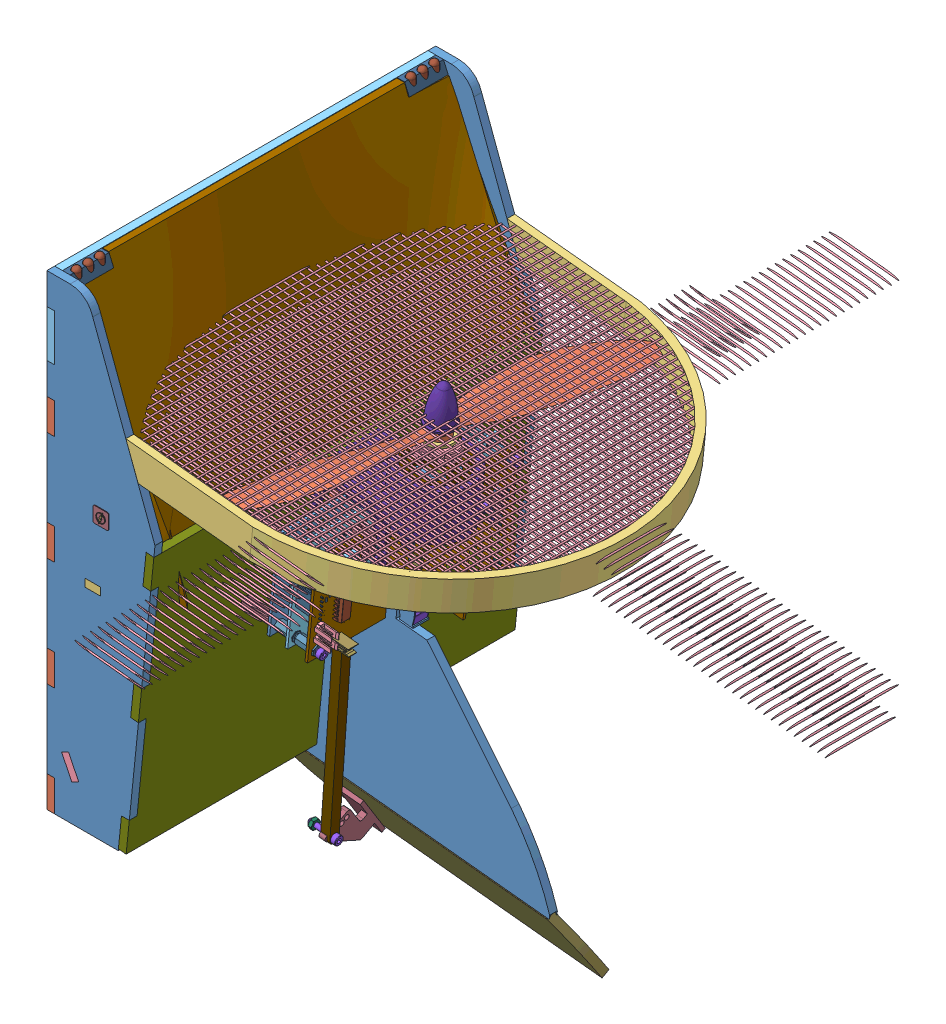
SolidWorks assembly AssTotaleSimu2, configuration Défaut. Lengths in mm. (continued)
Components (placement in the parent): (continued)
- AssStructSimu-1: AssStructSimu [Défaut] at (-125.7658 -1.8483 624.6548) x (1 0 0) z (0 0 -1) size (253.25 324.59 251.6) (continued)
  - AssProtec-1: AssProtec [Défaut] at (86.6746 190.4649 284.6351) x (0 0 -1) z (0.101852 -0.9948 0) size (250 237.46 20) (continued)
    - AssGrillage-2: AssGrillage [Défaut] at (339.6086 -132.5428 241.6839) x (0 0 1) z (-1 0 0) size (2.02 237.05 250) (continued)
      - barreau-208: barreau [Défaut] at (-0.1839 -1.5314 233.7823) x (0.998922 0 0.04641) z (0 1 0) size (1 1 400)
      - barreau-209: barreau [Défaut] at (-0.1839 -1.5314 228.7823) x (0.998922 0 0.04641) z (0 1 0) size (1 1 400)
      - barreau-210: barreau [Défaut] at (-0.1839 -1.5314 223.7823) x (0.998922 0 0.04641) z (0 1 0) size (1 1 400)
      - barreau-211: barreau [Défaut] at (-0.1839 -1.5314 218.7823) x (0.998922 0 0.04641) z (0 1 0) size (1 1 400)
      - barreau-212: barreau [Défaut] at (-0.1839 -1.5314 213.7823) x (0.998922 0 0.04641) z (0 1 0) size (1 1 400)
      - barreau-213: barreau [Défaut] at (-0.1839 -1.5314 208.7823) x (0.998922 0 0.04641) z (0 1 0) size (1 1 400)
      - barreau-214: barreau [Défaut] at (-0.1839 -1.5314 203.7823) x (0.998922 0 0.04641) z (0 1 0) size (1 1 400)
  - AssCarte-1: AssCarte [Défaut] at (38.0121 147.1029 290.772) x (-0.101852 0.9948 0) z (0.9948 0.101852 0) size (66.52 130.57 98.72)
    - carte_onduleur_v3-1: carte_onduleur_v3 [Défaut] at (-131.8199 12.0892 20.7912) size (66.52 130.57 82.34)
      - Layer_1-1: Layer_1 [Défaut] at origin size (60 130 1.61)
      - BTN-1: BTN [Défaut] at (-25.5 7.4 0.803) x (0 -1 0) z (0 0 1) size (6.76 3.64 4.37)
        - Open CASCADE STEP translator 6.8 1.2.1-1: Open CASCADE STEP translator 6.8 1.2.1 [Défaut] at origin size (6.76 3.64 4.37)
          - Body_1-1: Body_1 [Défaut] at (-0.5 -2 0) size (6.76 3.64 4.37)
            - =_[0_1_1_3]-1: =_[0_1_1_3] [Défaut] at origin size (6 3.64 4.37)
            - =_[0_1_1_4]-1: =_[0_1_1_4] [Défaut] at origin size (0.38 1 0.67)
            - =_[0_1_1_5]-1: =_[0_1_1_5] [Défaut] at origin size (0.38 1 0.67)
      - CON_IO1-1: CON_IO1 [Défaut] at (-11.3 12.1 0.803) x (0 -1 0) z (0 0 1) size (13 30 57.5)
        - Open CASCADE STEP translator 6.8 1.3.1-1: Open CASCADE STEP translator 6.8 1.3.1 [Défaut] at origin size (13 30 57.5)
          - Body_1_2-1: Body_1_2 [Défaut] at (-3 -15 8) x (0 -1 0) z (-1 0 0) size (30 57.5 13)
            - 1-1: 1 [Défaut] at origin size (30 50 1.61)
            - 10-1: 10 [Défaut] at (-14.395 31.0465 0.803) x (-1 0 0) z (0 0 1) size (5.59 6.35 1.11)
              - =_[0_1_1_4]-1: =_[0_1_1_4] [Défaut] at origin size (5.59 6.35 1.11)
                - 11-1: 11 [Défaut] at (2 3.3 0) x (-1 0 0) z (0 0 1) size (5.59 6.35 1.11)
                  - =_[0_1_1_3]_2-1: =_[0_1_1_3]_2 [Défaut] at origin size (0.44 0.55 0.36)
                  - =_[0_1_1_4]_2-1: =_[0_1_1_4]_2 [Défaut] at origin size (5.59 4.15 0.36)
                  - =_[0_1_1_5]_2-1: =_[0_1_1_5]_2 [Défaut] at origin size (5.35 6.1 1.1)
                  - =_[0_1_1_6]-1: =_[0_1_1_6] [Défaut] at origin size (0.44 0.55 0.36)
                  - =_[0_1_1_7]-1: =_[0_1_1_7] [Défaut] at origin size (0.44 0.55 0.36)
                  - =_[0_1_1_8]-1: =_[0_1_1_8] [Défaut] at origin size (0.44 0.55 0.36)
            - 13-1: 13 [Défaut] at (-12.62 16.6 -0.803) x (-1 0 0) z (0 0 -1) size (5.59 6.35 1.11)
              - =_[0_1_1_13]-1: =_[0_1_1_13] [Défaut] at origin size (5.59 6.35 1.11)
                - 11-1: 11 [Défaut] at (2 3.3 0) x (-1 0 0) z (0 0 1) size (5.59 6.35 1.11)
                  - =_[0_1_1_3]_2-1: =_[0_1_1_3]_2 [Défaut] at origin size (0.44 0.55 0.36)
                  - =_[0_1_1_4]_2-1: =_[0_1_1_4]_2 [Défaut] at origin size (5.59 4.15 0.36)
                  - =_[0_1_1_5]_2-1: =_[0_1_1_5]_2 [Défaut] at origin size (5.35 6.1 1.1)
                  - =_[0_1_1_6]-1: =_[0_1_1_6] [Défaut] at origin size (0.44 0.55 0.36)
                  - =_[0_1_1_7]-1: =_[0_1_1_7] [Défaut] at origin size (0.44 0.55 0.36)
                  - =_[0_1_1_8]-1: =_[0_1_1_8] [Défaut] at origin size (0.44 0.55 0.36)
            - 16-1: 16 [Défaut] at (-4.2 24.2 0.803) x (-1 0 0) z (0 0 1) size (12.8 0.5 13)
              - =_[0_1_1_15]-1: =_[0_1_1_15] [Défaut] at origin size (12.8 0.5 13)
                - 17-1: 17 [Défaut] at (2.7 0 0) x (1 0 0) z (0 -1 0) size (12.8 13 0.5)
            - 19-1: 19 [Défaut] at (-4.1 6.8 0.803) x (-1 0 0) z (0 0 1) size (12.8 0.5 13)
              - =_[0_1_1_18]-1: =_[0_1_1_18] [Défaut] at origin size (12.8 0.5 13)
                - 17-1: 17 [Défaut] at (2.7 0 0) x (1 0 0) z (0 -1 0) size (12.8 13 0.5)
            - 24-1: 24 [Défaut] at (-8.1 16.5 -0.803) x (0 1 0) z (0 0 -1) size (7.75 5.13 1.17)
              - =_[0_1_1_20]-1: =_[0_1_1_20] [Défaut] at origin size (7.75 5.13 1.17)
                - 20-1: 20 [Défaut] at origin size (7.59 5.13 1.07)
                - 21-1: 21 [Défaut] at (-14.478 0 0) x (-1 0 0) z (0 0 1) size (0.76 5.08 1.17)
                - 22-1: 22 [Défaut] at origin size (0.76 5.08 1.17)
            - 35-1: 35 [Défaut] at (-25.3 25.5 0.803) x (0 -1 0) z (0 0 1) size (6.05 5.2 1.7)
              - =_[0_1_1_25]-1: =_[0_1_1_25] [Défaut] at origin size (6.05 5.2 1.7)
                - 25-1: 25 [Défaut] at origin size (4.3 5.2 1.53)
                - 26-1: 26 [Défaut] at origin size (0.88 0.51 1.06)
                - 27-1: 27 [Défaut] at origin size (0.88 0.51 1.06)
                - 28-1: 28 [Défaut] at origin size (0.88 0.51 1.06)
                - 29-1: 29 [Défaut] at origin size (0.88 0.51 1.06)
                - 30-1: 30 [Défaut] at (11.6 -5.08 0) x (-1 0 0) z (0 0 1) size (0.87 0.51 1.06)
                - 31-1: 31 [Défaut] at (11.6 -2.54 0) x (-1 0 0) z (0 0 1) size (0.87 0.51 1.06)
                - 32-1: 32 [Défaut] at (11.6 0 0) x (-1 0 0) z (0 0 1) size (0.87 0.51 1.06)
                - 33-1: 33 [Défaut] at (11.6 2.54 0) x (-1 0 0) z (0 0 1) size (0.87 0.51 1.06)
            - 40-1: 40 [Défaut] at (-27.6 27.2 0.803) size (2.34 1.04 0.5)
              - =_[0_1_1_36]-1: =_[0_1_1_36] [Défaut] at origin size (2.34 1.04 0.5)
                - 36-1: 36 [Défaut] at origin size (2.29 1.04 0.43)
                - 37-1: 37 [Défaut] at (0.3048 0 0) x (-1 0 0) z (0 0 1) size (0.51 1.02 0.5)
                - 38-1: 38 [Défaut] at origin size (0.51 1.02 0.5)
            - 42-1: 42 [Défaut] at (-22.1 21.6 0.803) x (0 1 0) z (0 0 1) size (2.34 1.04 0.5)
              - =_[0_1_1_36]-1: =_[0_1_1_36] [Défaut] at origin size (2.34 1.04 0.5)
                - 36-1: 36 [Défaut] at origin size (2.29 1.04 0.43)
                - 37-1: 37 [Défaut] at (0.3048 0 0) x (-1 0 0) z (0 0 1) size (0.51 1.02 0.5)
                - 38-1: 38 [Défaut] at origin size (0.51 1.02 0.5)
            - 47-1: 47 [Défaut] at (-14.7664 14.5 -0.803) x (-1 0 0) z (0 0 -1) size (2.34 1.04 0.5)
              - =_[0_1_1_42]-1: =_[0_1_1_42] [Défaut] at origin size (2.34 1.04 0.5)
                - 43-1: 43 [Défaut] at origin size (2.29 1.04 0.43)
                - 44-1: 44 [Défaut] at (0.3048 0 0) x (-1 0 0) z (0 0 1) size (0.51 1.02 0.5)
                - 45-1: 45 [Défaut] at origin size (0.51 1.02 0.5)
            - 57-1: 57 [Défaut] at (-15.3 2.7 -0.803) x (0 -1 0) z (0 0 -1) size (10.36 15.24 6.14)
              - =_[0_1_1_47]-1: =_[0_1_1_47] [Défaut] at origin size (10.36 15.24 6.14)
                - 55-1: 55 [Défaut] at (1.8 -1.2 3) x (1 0 0) z (0 1 0) size (10.36 6.14 15.24)
                  - 54-1: 54 [Défaut] at origin size (10.36 6.14 7.62)
                    - 52-1: 52 [Défaut] at origin size (10.36 6.14 2.54)
                      - 48-1: 48 [Défaut] at origin size (8.4 2.54 2.54)
                      - 49-1: 49 [Défaut] at (-0.0461 1.2682 1.27) x (0 0 -1) z (0.999998 -0.002105 0) size (1.95 5.07 7.58)
                    - 52-2: 52 [Défaut] at (0 0 -2.54) size (10.36 6.14 2.54)
                      - 48-1: 48 [Défaut] at origin size (8.4 2.54 2.54)
                      - 49-1: 49 [Défaut] at (-0.0461 1.2682 1.27) x (0 0 -1) z (0.999998 -0.002105 0) size (1.95 5.07 7.58)
                    - 52-3: 52 [Défaut] at (0 0 -5.08) size (10.36 6.14 2.54)
                      - 48-1: 48 [Défaut] at origin size (8.4 2.54 2.54)
                      - 49-1: 49 [Défaut] at (-0.0461 1.2682 1.27) x (0 0 -1) z (0.999998 -0.002105 0) size (1.95 5.07 7.58)
                  - 54-2: 54 [Défaut] at (0 0 -7.62) size (10.36 6.14 7.62)
                    - 52-1: 52 [Défaut] at origin size (10.36 6.14 2.54)
                      - 48-1: 48 [Défaut] at origin size (8.4 2.54 2.54)
                      - 49-1: 49 [Défaut] at (-0.0461 1.2682 1.27) x (0 0 -1) z (0.999998 -0.002105 0) size (1.95 5.07 7.58)
                    - 52-2: 52 [Défaut] at (0 0 -2.54) size (10.36 6.14 2.54)
                      - 48-1: 48 [Défaut] at origin size (8.4 2.54 2.54)
                      - 49-1: 49 [Défaut] at (-0.0461 1.2682 1.27) x (0 0 -1) z (0.999998 -0.002105 0) size (1.95 5.07 7.58)
                    - 52-3: 52 [Défaut] at (0 0 -5.08) size (10.36 6.14 2.54)
                      - 48-1: 48 [Défaut] at origin size (8.4 2.54 2.54)
                      - 49-1: 49 [Défaut] at (-0.0461 1.2682 1.27) x (0 0 -1) z (0.999998 -0.002105 0) size (1.95 5.07 7.58)
            - 59-1: 59 [Défaut] at (-26.5 31 0.803) x (0 -1 0) z (0 0 1) size (2.34 1.04 0.5)
              - =_[0_1_1_42]-1: =_[0_1_1_42] [Défaut] at origin size (2.34 1.04 0.5)
                - 43-1: 43 [Défaut] at origin size (2.29 1.04 0.43)
                - 44-1: 44 [Défaut] at (0.3048 0 0) x (-1 0 0) z (0 0 1) size (0.51 1.02 0.5)
                - 45-1: 45 [Défaut] at origin size (0.51 1.02 0.5)
            - 61-1: 61 [Défaut] at (-21.6 17.8 0.803) x (-1 0 0) z (0 0 1) size (2.34 1.04 0.5)
              - =_[0_1_1_42]-1: =_[0_1_1_42] [Défaut] at origin size (2.34 1.04 0.5)
                - 43-1: 43 [Défaut] at origin size (2.29 1.04 0.43)
                - 44-1: 44 [Défaut] at (0.3048 0 0) x (-1 0 0) z (0 0 1) size (0.51 1.02 0.5)
                - 45-1: 45 [Défaut] at origin size (0.51 1.02 0.5)
            - 74-1: 74 [Défaut] at (-4.9 41.8 0.803) x (0 -1 0) z (0 0 1) size (6 4.9 1.75)
              - =_[0_1_1_56]-1: =_[0_1_1_56] [Défaut] at origin size (6 4.9 1.75)
                - 72-1: 72 [Défaut] at origin size (6 4.9 1.75)
                  - =_[0_1_1_2]-1: =_[0_1_1_2] [Défaut] at origin size (3.9 4.9 1.57)
                  - =_[0_1_1_3]-1: =_[0_1_1_3] [Défaut] at origin size (6 4.22 1)
                    - =_[0_1_1_60]-1: =_[0_1_1_60] [Défaut] at origin size (1.05 0.41 1)
                    - =_[0_1_1_61]-1: =_[0_1_1_61] [Défaut] at origin size (1.05 0.41 1)
                    - =_[0_1_1_62]-1: =_[0_1_1_62] [Défaut] at origin size (1.05 0.41 1)
                    - =_[0_1_1_63]-1: =_[0_1_1_63] [Défaut] at origin size (1.05 0.41 1)
                    - =_[0_1_1_64]-1: =_[0_1_1_64] [Défaut] at origin size (1.05 0.41 1)
                    - =_[0_1_1_65]-1: =_[0_1_1_65] [Défaut] at origin size (1.05 0.41 1)
                    - =_[0_1_1_66]-1: =_[0_1_1_66] [Défaut] at origin size (1.05 0.41 1)
                    - =_[0_1_1_67]-1: =_[0_1_1_67] [Défaut] at origin size (1.05 0.41 1)
            - 76-1: 76 [Défaut] at (-8.5 40.5664 0.803) x (0 1 0) z (0 0 1) size (2.34 1.04 0.5)
              - =_[0_1_1_42]-1: =_[0_1_1_42] [Défaut] at origin size (2.34 1.04 0.5)
                - 43-1: 43 [Défaut] at origin size (2.29 1.04 0.43)
                - 44-1: 44 [Défaut] at (0.3048 0 0) x (-1 0 0) z (0 0 1) size (0.51 1.02 0.5)
                - 45-1: 45 [Défaut] at origin size (0.51 1.02 0.5)
            - 78-1: 78 [Défaut] at (-5.9 46.4 0.803) x (-1 0 0) z (0 0 1) size (2.34 1.04 0.5)
              - =_[0_1_1_42]-1: =_[0_1_1_42] [Défaut] at origin size (2.34 1.04 0.5)
                - 43-1: 43 [Défaut] at origin size (2.29 1.04 0.43)
                - 44-1: 44 [Défaut] at (0.3048 0 0) x (-1 0 0) z (0 0 1) size (0.51 1.02 0.5)
                - 45-1: 45 [Défaut] at origin size (0.51 1.02 0.5)
            - 80-1: 80 [Défaut] at (-7 48.1 0.803) size (2.34 1.04 0.5)
              - =_[0_1_1_42]-1: =_[0_1_1_42] [Défaut] at origin size (2.34 1.04 0.5)
                - 43-1: 43 [Défaut] at origin size (2.29 1.04 0.43)
                - 44-1: 44 [Défaut] at (0.3048 0 0) x (-1 0 0) z (0 0 1) size (0.51 1.02 0.5)
                - 45-1: 45 [Défaut] at origin size (0.51 1.02 0.5)
            - 82-1: 82 [Défaut] at (-6 37.1 0.803) size (2.34 1.04 0.5)
              - =_[0_1_1_42]-1: =_[0_1_1_42] [Défaut] at origin size (2.34 1.04 0.5)
                - 43-1: 43 [Défaut] at origin size (2.29 1.04 0.43)
                - 44-1: 44 [Défaut] at (0.3048 0 0) x (-1 0 0) z (0 0 1) size (0.51 1.02 0.5)
                - 45-1: 45 [Défaut] at origin size (0.51 1.02 0.5)
      - CON_IO2-1: CON_IO2 [Défaut] at (-11.3 -2.7 0.803) x (0 -1 0) z (0 0 1) size (13 30 57.5)
        - Open CASCADE STEP translator 6.8 1.4.1-1: Open CASCADE STEP translator 6.8 1.4.1 [Défaut] at origin size (13 30 57.5)
          - Body_1_2-1: Body_1_2 [Défaut] at (-3 -15 8) x (0 -1 0) z (-1 0 0) size (30 57.5 13)
            - 1-1: 1 [Défaut] at origin size (30 50 1.61)
            - 10-1: 10 [Défaut] at (-14.395 31.0465 0.803) x (-1 0 0) z (0 0 1) size (5.59 6.35 1.11)
              - =_[0_1_1_4]-1: =_[0_1_1_4] [Défaut] at origin size (5.59 6.35 1.11)
                - 11-1: 11 [Défaut] at (2 3.3 0) x (-1 0 0) z (0 0 1) size (5.59 6.35 1.11)
                  - =_[0_1_1_3]_2-1: =_[0_1_1_3]_2 [Défaut] at origin size (0.44 0.55 0.36)
                  - =_[0_1_1_4]_2-1: =_[0_1_1_4]_2 [Défaut] at origin size (5.59 4.15 0.36)
                  - =_[0_1_1_5]_2-1: =_[0_1_1_5]_2 [Défaut] at origin size (5.35 6.1 1.1)
                  - =_[0_1_1_6]-1: =_[0_1_1_6] [Défaut] at origin size (0.44 0.55 0.36)
                  - =_[0_1_1_7]-1: =_[0_1_1_7] [Défaut] at origin size (0.44 0.55 0.36)
                  - =_[0_1_1_8]-1: =_[0_1_1_8] [Défaut] at origin size (0.44 0.55 0.36)
            - 13-1: 13 [Défaut] at (-12.62 16.6 -0.803) x (-1 0 0) z (0 0 -1) size (5.59 6.35 1.11)
              - =_[0_1_1_13]-1: =_[0_1_1_13] [Défaut] at origin size (5.59 6.35 1.11)
                - 11-1: 11 [Défaut] at (2 3.3 0) x (-1 0 0) z (0 0 1) size (5.59 6.35 1.11)
                  - =_[0_1_1_3]_2-1: =_[0_1_1_3]_2 [Défaut] at origin size (0.44 0.55 0.36)
                  - =_[0_1_1_4]_2-1: =_[0_1_1_4]_2 [Défaut] at origin size (5.59 4.15 0.36)
                  - =_[0_1_1_5]_2-1: =_[0_1_1_5]_2 [Défaut] at origin size (5.35 6.1 1.1)
                  - =_[0_1_1_6]-1: =_[0_1_1_6] [Défaut] at origin size (0.44 0.55 0.36)
                  - =_[0_1_1_7]-1: =_[0_1_1_7] [Défaut] at origin size (0.44 0.55 0.36)
                  - =_[0_1_1_8]-1: =_[0_1_1_8] [Défaut] at origin size (0.44 0.55 0.36)
            - 16-1: 16 [Défaut] at (-4.2 24.2 0.803) x (-1 0 0) z (0 0 1) size (12.8 0.5 13)
              - =_[0_1_1_15]-1: =_[0_1_1_15] [Défaut] at origin size (12.8 0.5 13)
                - 17-1: 17 [Défaut] at (2.7 0 0) x (1 0 0) z (0 -1 0) size (12.8 13 0.5)
            - 19-1: 19 [Défaut] at (-4.1 6.8 0.803) x (-1 0 0) z (0 0 1) size (12.8 0.5 13)
              - =_[0_1_1_18]-1: =_[0_1_1_18] [Défaut] at origin size (12.8 0.5 13)
                - 17-1: 17 [Défaut] at (2.7 0 0) x (1 0 0) z (0 -1 0) size (12.8 13 0.5)
            - 24-1: 24 [Défaut] at (-8.1 16.5 -0.803) x (0 1 0) z (0 0 -1) size (7.75 5.13 1.17)
              - =_[0_1_1_20]-1: =_[0_1_1_20] [Défaut] at origin size (7.75 5.13 1.17)
                - 20-1: 20 [Défaut] at origin size (7.59 5.13 1.07)
                - 21-1: 21 [Défaut] at (-14.478 0 0) x (-1 0 0) z (0 0 1) size (0.76 5.08 1.17)
                - 22-1: 22 [Défaut] at origin size (0.76 5.08 1.17)
            - 35-1: 35 [Défaut] at (-25.3 25.5 0.803) x (0 -1 0) z (0 0 1) size (6.05 5.2 1.7)
              - =_[0_1_1_25]-1: =_[0_1_1_25] [Défaut] at origin size (6.05 5.2 1.7)
                - 25-1: 25 [Défaut] at origin size (4.3 5.2 1.53)
                - 26-1: 26 [Défaut] at origin size (0.88 0.51 1.06)
                - 27-1: 27 [Défaut] at origin size (0.88 0.51 1.06)
                - 28-1: 28 [Défaut] at origin size (0.88 0.51 1.06)
                - 29-1: 29 [Défaut] at origin size (0.88 0.51 1.06)
                - 30-1: 30 [Défaut] at (11.6 -5.08 0) x (-1 0 0) z (0 0 1) size (0.87 0.51 1.06)
                - 31-1: 31 [Défaut] at (11.6 -2.54 0) x (-1 0 0) z (0 0 1) size (0.87 0.51 1.06)
                - 32-1: 32 [Défaut] at (11.6 0 0) x (-1 0 0) z (0 0 1) size (0.87 0.51 1.06)
                - 33-1: 33 [Défaut] at (11.6 2.54 0) x (-1 0 0) z (0 0 1) size (0.87 0.51 1.06)
            - 40-1: 40 [Défaut] at (-27.6 27.2 0.803) size (2.34 1.04 0.5)
              - =_[0_1_1_36]-1: =_[0_1_1_36] [Défaut] at origin size (2.34 1.04 0.5)
                - 36-1: 36 [Défaut] at origin size (2.29 1.04 0.43)
                - 37-1: 37 [Défaut] at (0.3048 0 0) x (-1 0 0) z (0 0 1) size (0.51 1.02 0.5)
                - 38-1: 38 [Défaut] at origin size (0.51 1.02 0.5)
            - 42-1: 42 [Défaut] at (-22.1 21.6 0.803) x (0 1 0) z (0 0 1) size (2.34 1.04 0.5)
              - =_[0_1_1_36]-1: =_[0_1_1_36] [Défaut] at origin size (2.34 1.04 0.5)
                - 36-1: 36 [Défaut] at origin size (2.29 1.04 0.43)
                - 37-1: 37 [Défaut] at (0.3048 0 0) x (-1 0 0) z (0 0 1) size (0.51 1.02 0.5)
                - 38-1: 38 [Défaut] at origin size (0.51 1.02 0.5)
            - 47-1: 47 [Défaut] at (-14.7664 14.5 -0.803) x (-1 0 0) z (0 0 -1) size (2.34 1.04 0.5)
              - =_[0_1_1_42]-1: =_[0_1_1_42] [Défaut] at origin size (2.34 1.04 0.5)
                - 43-1: 43 [Défaut] at origin size (2.29 1.04 0.43)
                - 44-1: 44 [Défaut] at (0.3048 0 0) x (-1 0 0) z (0 0 1) size (0.51 1.02 0.5)
                - 45-1: 45 [Défaut] at origin size (0.51 1.02 0.5)
            - 57-1: 57 [Défaut] at (-15.3 2.7 -0.803) x (0 -1 0) z (0 0 -1) size (10.36 15.24 6.14)
              - =_[0_1_1_47]-1: =_[0_1_1_47] [Défaut] at origin size (10.36 15.24 6.14)
                - 55-1: 55 [Défaut] at (1.8 -1.2 3) x (1 0 0) z (0 1 0) size (10.36 6.14 15.24)
                  - 54-1: 54 [Défaut] at origin size (10.36 6.14 7.62)
                    - 52-1: 52 [Défaut] at origin size (10.36 6.14 2.54)
                      - 48-1: 48 [Défaut] at origin size (8.4 2.54 2.54)
                      - 49-1: 49 [Défaut] at (-0.0461 1.2682 1.27) x (0 0 -1) z (0.999998 -0.002105 0) size (1.95 5.07 7.58)
                    - 52-2: 52 [Défaut] at (0 0 -2.54) size (10.36 6.14 2.54)
                      - 48-1: 48 [Défaut] at origin size (8.4 2.54 2.54)
                      - 49-1: 49 [Défaut] at (-0.0461 1.2682 1.27) x (0 0 -1) z (0.999998 -0.002105 0) size (1.95 5.07 7.58)
                    - 52-3: 52 [Défaut] at (0 0 -5.08) size (10.36 6.14 2.54)
                      - 48-1: 48 [Défaut] at origin size (8.4 2.54 2.54)
                      - 49-1: 49 [Défaut] at (-0.0461 1.2682 1.27) x (0 0 -1) z (0.999998 -0.002105 0) size (1.95 5.07 7.58)
                  - 54-2: 54 [Défaut] at (0 0 -7.62) size (10.36 6.14 7.62)
                    - 52-1: 52 [Défaut] at origin size (10.36 6.14 2.54)
                      - 48-1: 48 [Défaut] at origin size (8.4 2.54 2.54)
                      - 49-1: 49 [Défaut] at (-0.0461 1.2682 1.27) x (0 0 -1) z (0.999998 -0.002105 0) size (1.95 5.07 7.58)
                    - 52-2: 52 [Défaut] at (0 0 -2.54) size (10.36 6.14 2.54)
                      - 48-1: 48 [Défaut] at origin size (8.4 2.54 2.54)
                      - 49-1: 49 [Défaut] at (-0.0461 1.2682 1.27) x (0 0 -1) z (0.999998 -0.002105 0) size (1.95 5.07 7.58)
                    - 52-3: 52 [Défaut] at (0 0 -5.08) size (10.36 6.14 2.54)
                      - 48-1: 48 [Défaut] at origin size (8.4 2.54 2.54)
                      - 49-1: 49 [Défaut] at (-0.0461 1.2682 1.27) x (0 0 -1) z (0.999998 -0.002105 0) size (1.95 5.07 7.58)
            - 59-1: 59 [Défaut] at (-26.5 31 0.803) x (0 -1 0) z (0 0 1) size (2.34 1.04 0.5)
              - =_[0_1_1_42]-1: =_[0_1_1_42] [Défaut] at origin size (2.34 1.04 0.5)
                - 43-1: 43 [Défaut] at origin size (2.29 1.04 0.43)
                - 44-1: 44 [Défaut] at (0.3048 0 0) x (-1 0 0) z (0 0 1) size (0.51 1.02 0.5)
                - 45-1: 45 [Défaut] at origin size (0.51 1.02 0.5)
            - 61-1: 61 [Défaut] at (-21.6 17.8 0.803) x (-1 0 0) z (0 0 1) size (2.34 1.04 0.5)
              - =_[0_1_1_42]-1: =_[0_1_1_42] [Défaut] at origin size (2.34 1.04 0.5)
                - 43-1: 43 [Défaut] at origin size (2.29 1.04 0.43)
                - 44-1: 44 [Défaut] at (0.3048 0 0) x (-1 0 0) z (0 0 1) size (0.51 1.02 0.5)
                - 45-1: 45 [Défaut] at origin size (0.51 1.02 0.5)
            - 74-1: 74 [Défaut] at (-4.9 41.8 0.803) x (0 -1 0) z (0 0 1) size (6 4.9 1.75)
              - =_[0_1_1_56]-1: =_[0_1_1_56] [Défaut] at origin size (6 4.9 1.75)
                - 72-1: 72 [Défaut] at origin size (6 4.9 1.75)
                  - =_[0_1_1_2]-1: =_[0_1_1_2] [Défaut] at origin size (3.9 4.9 1.57)
                  - =_[0_1_1_3]-1: =_[0_1_1_3] [Défaut] at origin size (6 4.22 1)
                    - =_[0_1_1_60]-1: =_[0_1_1_60] [Défaut] at origin size (1.05 0.41 1)
                    - =_[0_1_1_61]-1: =_[0_1_1_61] [Défaut] at origin size (1.05 0.41 1)
                    - =_[0_1_1_62]-1: =_[0_1_1_62] [Défaut] at origin size (1.05 0.41 1)
                    - =_[0_1_1_63]-1: =_[0_1_1_63] [Défaut] at origin size (1.05 0.41 1)
                    - =_[0_1_1_64]-1: =_[0_1_1_64] [Défaut] at origin size (1.05 0.41 1)
                    - =_[0_1_1_65]-1: =_[0_1_1_65] [Défaut] at origin size (1.05 0.41 1)
                    - =_[0_1_1_66]-1: =_[0_1_1_66] [Défaut] at origin size (1.05 0.41 1)
                    - =_[0_1_1_67]-1: =_[0_1_1_67] [Défaut] at origin size (1.05 0.41 1)
            - 76-1: 76 [Défaut] at (-8.5 40.5664 0.803) x (0 1 0) z (0 0 1) size (2.34 1.04 0.5)
              - =_[0_1_1_42]-1: =_[0_1_1_42] [Défaut] at origin size (2.34 1.04 0.5)
                - 43-1: 43 [Défaut] at origin size (2.29 1.04 0.43)
                - 44-1: 44 [Défaut] at (0.3048 0 0) x (-1 0 0) z (0 0 1) size (0.51 1.02 0.5)
                - 45-1: 45 [Défaut] at origin size (0.51 1.02 0.5)
            - 78-1: 78 [Défaut] at (-5.9 46.4 0.803) x (-1 0 0) z (0 0 1) size (2.34 1.04 0.5)
              - =_[0_1_1_42]-1: =_[0_1_1_42] [Défaut] at origin size (2.34 1.04 0.5)
                - 43-1: 43 [Défaut] at origin size (2.29 1.04 0.43)
                - 44-1: 44 [Défaut] at (0.3048 0 0) x (-1 0 0) z (0 0 1) size (0.51 1.02 0.5)
                - 45-1: 45 [Défaut] at origin size (0.51 1.02 0.5)
            - 80-1: 80 [Défaut] at (-7 48.1 0.803) size (2.34 1.04 0.5)
              - =_[0_1_1_42]-1: =_[0_1_1_42] [Défaut] at origin size (2.34 1.04 0.5)
                - 43-1: 43 [Défaut] at origin size (2.29 1.04 0.43)
                - 44-1: 44 [Défaut] at (0.3048 0 0) x (-1 0 0) z (0 0 1) size (0.51 1.02 0.5)
                - 45-1: 45 [Défaut] at origin size (0.51 1.02 0.5)
            - 82-1: 82 [Défaut] at (-6 37.1 0.803) size (2.34 1.04 0.5)
              - =_[0_1_1_42]-1: =_[0_1_1_42] [Défaut] at origin size (2.34 1.04 0.5)
                - 43-1: 43 [Défaut] at origin size (2.29 1.04 0.43)
                - 44-1: 44 [Défaut] at (0.3048 0 0) x (-1 0 0) z (0 0 1) size (0.51 1.02 0.5)
                - 45-1: 45 [Défaut] at origin size (0.51 1.02 0.5)
      - CON_IO3-1: CON_IO3 [Défaut] at (-11.3 -17.7 0.803) x (0 -1 0) z (0 0 1) size (13 30 57.5)
        - Open CASCADE STEP translator 6.8 1.5.1-1: Open CASCADE STEP translator 6.8 1.5.1 [Défaut] at origin size (13 30 57.5)
          - Body_1_2-1: Body_1_2 [Défaut] at (-3 -15 8) x (0 -1 0) z (-1 0 0) size (30 57.5 13)
            - 1-1: 1 [Défaut] at origin size (30 50 1.61)
            - 10-1: 10 [Défaut] at (-14.395 31.0465 0.803) x (-1 0 0) z (0 0 1) size (5.59 6.35 1.11)
              - =_[0_1_1_4]-1: =_[0_1_1_4] [Défaut] at origin size (5.59 6.35 1.11)
                - 11-1: 11 [Défaut] at (2 3.3 0) x (-1 0 0) z (0 0 1) size (5.59 6.35 1.11)
                  - =_[0_1_1_3]_2-1: =_[0_1_1_3]_2 [Défaut] at origin size (0.44 0.55 0.36)
                  - =_[0_1_1_4]_2-1: =_[0_1_1_4]_2 [Défaut] at origin size (5.59 4.15 0.36)
                  - =_[0_1_1_5]_2-1: =_[0_1_1_5]_2 [Défaut] at origin size (5.35 6.1 1.1)
                  - =_[0_1_1_6]-1: =_[0_1_1_6] [Défaut] at origin size (0.44 0.55 0.36)
                  - =_[0_1_1_7]-1: =_[0_1_1_7] [Défaut] at origin size (0.44 0.55 0.36)
                  - =_[0_1_1_8]-1: =_[0_1_1_8] [Défaut] at origin size (0.44 0.55 0.36)
            - 13-1: 13 [Défaut] at (-12.62 16.6 -0.803) x (-1 0 0) z (0 0 -1) size (5.59 6.35 1.11)
              - =_[0_1_1_13]-1: =_[0_1_1_13] [Défaut] at origin size (5.59 6.35 1.11)
                - 11-1: 11 [Défaut] at (2 3.3 0) x (-1 0 0) z (0 0 1) size (5.59 6.35 1.11)
                  - =_[0_1_1_3]_2-1: =_[0_1_1_3]_2 [Défaut] at origin size (0.44 0.55 0.36)
                  - =_[0_1_1_4]_2-1: =_[0_1_1_4]_2 [Défaut] at origin size (5.59 4.15 0.36)
                  - =_[0_1_1_5]_2-1: =_[0_1_1_5]_2 [Défaut] at origin size (5.35 6.1 1.1)
                  - =_[0_1_1_6]-1: =_[0_1_1_6] [Défaut] at origin size (0.44 0.55 0.36)
                  - =_[0_1_1_7]-1: =_[0_1_1_7] [Défaut] at origin size (0.44 0.55 0.36)
                  - =_[0_1_1_8]-1: =_[0_1_1_8] [Défaut] at origin size (0.44 0.55 0.36)
            - 16-1: 16 [Défaut] at (-4.2 24.2 0.803) x (-1 0 0) z (0 0 1) size (12.8 0.5 13)
              - =_[0_1_1_15]-1: =_[0_1_1_15] [Défaut] at origin size (12.8 0.5 13)
                - 17-1: 17 [Défaut] at (2.7 0 0) x (1 0 0) z (0 -1 0) size (12.8 13 0.5)
            - 19-1: 19 [Défaut] at (-4.1 6.8 0.803) x (-1 0 0) z (0 0 1) size (12.8 0.5 13)
              - =_[0_1_1_18]-1: =_[0_1_1_18] [Défaut] at origin size (12.8 0.5 13)
                - 17-1: 17 [Défaut] at (2.7 0 0) x (1 0 0) z (0 -1 0) size (12.8 13 0.5)
            - 24-1: 24 [Défaut] at (-8.1 16.5 -0.803) x (0 1 0) z (0 0 -1) size (7.75 5.13 1.17)
              - =_[0_1_1_20]-1: =_[0_1_1_20] [Défaut] at origin size (7.75 5.13 1.17)
                - 20-1: 20 [Défaut] at origin size (7.59 5.13 1.07)
                - 21-1: 21 [Défaut] at (-14.478 0 0) x (-1 0 0) z (0 0 1) size (0.76 5.08 1.17)
                - 22-1: 22 [Défaut] at origin size (0.76 5.08 1.17)
            - 35-1: 35 [Défaut] at (-25.3 25.5 0.803) x (0 -1 0) z (0 0 1) size (6.05 5.2 1.7)
              - =_[0_1_1_25]-1: =_[0_1_1_25] [Défaut] at origin size (6.05 5.2 1.7)
                - 25-1: 25 [Défaut] at origin size (4.3 5.2 1.53)
                - 26-1: 26 [Défaut] at origin size (0.88 0.51 1.06)
                - 27-1: 27 [Défaut] at origin size (0.88 0.51 1.06)
                - 28-1: 28 [Défaut] at origin size (0.88 0.51 1.06)
                - 29-1: 29 [Défaut] at origin size (0.88 0.51 1.06)
                - 30-1: 30 [Défaut] at (11.6 -5.08 0) x (-1 0 0) z (0 0 1) size (0.87 0.51 1.06)
                - 31-1: 31 [Défaut] at (11.6 -2.54 0) x (-1 0 0) z (0 0 1) size (0.87 0.51 1.06)
                - 32-1: 32 [Défaut] at (11.6 0 0) x (-1 0 0) z (0 0 1) size (0.87 0.51 1.06)
                - 33-1: 33 [Défaut] at (11.6 2.54 0) x (-1 0 0) z (0 0 1) size (0.87 0.51 1.06)
            - 40-1: 40 [Défaut] at (-27.6 27.2 0.803) size (2.34 1.04 0.5)
              - =_[0_1_1_36]-1: =_[0_1_1_36] [Défaut] at origin size (2.34 1.04 0.5)
                - 36-1: 36 [Défaut] at origin size (2.29 1.04 0.43)
                - 37-1: 37 [Défaut] at (0.3048 0 0) x (-1 0 0) z (0 0 1) size (0.51 1.02 0.5)
                - 38-1: 38 [Défaut] at origin size (0.51 1.02 0.5)
            - 42-1: 42 [Défaut] at (-22.1 21.6 0.803) x (0 1 0) z (0 0 1) size (2.34 1.04 0.5)
              - =_[0_1_1_36]-1: =_[0_1_1_36] [Défaut] at origin size (2.34 1.04 0.5)
                - 36-1: 36 [Défaut] at origin size (2.29 1.04 0.43)
                - 37-1: 37 [Défaut] at (0.3048 0 0) x (-1 0 0) z (0 0 1) size (0.51 1.02 0.5)
                - 38-1: 38 [Défaut] at origin size (0.51 1.02 0.5)
            - 47-1: 47 [Défaut] at (-14.7664 14.5 -0.803) x (-1 0 0) z (0 0 -1) size (2.34 1.04 0.5)
              - =_[0_1_1_42]-1: =_[0_1_1_42] [Défaut] at origin size (2.34 1.04 0.5)
                - 43-1: 43 [Défaut] at origin size (2.29 1.04 0.43)
                - 44-1: 44 [Défaut] at (0.3048 0 0) x (-1 0 0) z (0 0 1) size (0.51 1.02 0.5)
                - 45-1: 45 [Défaut] at origin size (0.51 1.02 0.5)
            - 57-1: 57 [Défaut] at (-15.3 2.7 -0.803) x (0 -1 0) z (0 0 -1) size (10.36 15.24 6.14)
              - =_[0_1_1_47]-1: =_[0_1_1_47] [Défaut] at origin size (10.36 15.24 6.14)
                - 55-1: 55 [Défaut] at (1.8 -1.2 3) x (1 0 0) z (0 1 0) size (10.36 6.14 15.24)
                  - 54-1: 54 [Défaut] at origin size (10.36 6.14 7.62)
                    - 52-1: 52 [Défaut] at origin size (10.36 6.14 2.54)
                      - 48-1: 48 [Défaut] at origin size (8.4 2.54 2.54)
                      - 49-1: 49 [Défaut] at (-0.0461 1.2682 1.27) x (0 0 -1) z (0.999998 -0.002105 0) size (1.95 5.07 7.58)
                    - 52-2: 52 [Défaut] at (0 0 -2.54) size (10.36 6.14 2.54)
                      - 48-1: 48 [Défaut] at origin size (8.4 2.54 2.54)
                      - 49-1: 49 [Défaut] at (-0.0461 1.2682 1.27) x (0 0 -1) z (0.999998 -0.002105 0) size (1.95 5.07 7.58)
                    - 52-3: 52 [Défaut] at (0 0 -5.08) size (10.36 6.14 2.54)
                      - 48-1: 48 [Défaut] at origin size (8.4 2.54 2.54)
                      - 49-1: 49 [Défaut] at (-0.0461 1.2682 1.27) x (0 0 -1) z (0.999998 -0.002105 0) size (1.95 5.07 7.58)
                  - 54-2: 54 [Défaut] at (0 0 -7.62) size (10.36 6.14 7.62)
                    - 52-1: 52 [Défaut] at origin size (10.36 6.14 2.54)
                      - 48-1: 48 [Défaut] at origin size (8.4 2.54 2.54)
                      - 49-1: 49 [Défaut] at (-0.0461 1.2682 1.27) x (0 0 -1) z (0.999998 -0.002105 0) size (1.95 5.07 7.58)
                    - 52-2: 52 [Défaut] at (0 0 -2.54) size (10.36 6.14 2.54)
                      - 48-1: 48 [Défaut] at origin size (8.4 2.54 2.54)
                      - 49-1: 49 [Défaut] at (-0.0461 1.2682 1.27) x (0 0 -1) z (0.999998 -0.002105 0) size (1.95 5.07 7.58)
                    - 52-3: 52 [Défaut] at (0 0 -5.08) size (10.36 6.14 2.54)
                      - 48-1: 48 [Défaut] at origin size (8.4 2.54 2.54)
                      - 49-1: 49 [Défaut] at (-0.0461 1.2682 1.27) x (0 0 -1) z (0.999998 -0.002105 0) size (1.95 5.07 7.58)
            - 59-1: 59 [Défaut] at (-26.5 31 0.803) x (0 -1 0) z (0 0 1) size (2.34 1.04 0.5)
              - =_[0_1_1_42]-1: =_[0_1_1_42] [Défaut] at origin size (2.34 1.04 0.5)
                - 43-1: 43 [Défaut] at origin size (2.29 1.04 0.43)
                - 44-1: 44 [Défaut] at (0.3048 0 0) x (-1 0 0) z (0 0 1) size (0.51 1.02 0.5)
                - 45-1: 45 [Défaut] at origin size (0.51 1.02 0.5)
            - 61-1: 61 [Défaut] at (-21.6 17.8 0.803) x (-1 0 0) z (0 0 1) size (2.34 1.04 0.5)
              - =_[0_1_1_42]-1: =_[0_1_1_42] [Défaut] at origin size (2.34 1.04 0.5)
                - 43-1: 43 [Défaut] at origin size (2.29 1.04 0.43)
                - 44-1: 44 [Défaut] at (0.3048 0 0) x (-1 0 0) z (0 0 1) size (0.51 1.02 0.5)
                - 45-1: 45 [Défaut] at origin size (0.51 1.02 0.5)
            - 74-1: 74 [Défaut] at (-4.9 41.8 0.803) x (0 -1 0) z (0 0 1) size (6 4.9 1.75)
              - =_[0_1_1_56]-1: =_[0_1_1_56] [Défaut] at origin size (6 4.9 1.75)
                - 72-1: 72 [Défaut] at origin size (6 4.9 1.75)
                  - =_[0_1_1_2]-1: =_[0_1_1_2] [Défaut] at origin size (3.9 4.9 1.57)
                  - =_[0_1_1_3]-1: =_[0_1_1_3] [Défaut] at origin size (6 4.22 1)
                    - =_[0_1_1_60]-1: =_[0_1_1_60] [Défaut] at origin size (1.05 0.41 1)
                    - =_[0_1_1_61]-1: =_[0_1_1_61] [Défaut] at origin size (1.05 0.41 1)
                    - =_[0_1_1_62]-1: =_[0_1_1_62] [Défaut] at origin size (1.05 0.41 1)
                    - =_[0_1_1_63]-1: =_[0_1_1_63] [Défaut] at origin size (1.05 0.41 1)
                    - =_[0_1_1_64]-1: =_[0_1_1_64] [Défaut] at origin size (1.05 0.41 1)
                    - =_[0_1_1_65]-1: =_[0_1_1_65] [Défaut] at origin size (1.05 0.41 1)
                    - =_[0_1_1_66]-1: =_[0_1_1_66] [Défaut] at origin size (1.05 0.41 1)
                    - =_[0_1_1_67]-1: =_[0_1_1_67] [Défaut] at origin size (1.05 0.41 1)
            - 76-1: 76 [Défaut] at (-8.5 40.5664 0.803) x (0 1 0) z (0 0 1) size (2.34 1.04 0.5)
              - =_[0_1_1_42]-1: =_[0_1_1_42] [Défaut] at origin size (2.34 1.04 0.5)
                - 43-1: 43 [Défaut] at origin size (2.29 1.04 0.43)
                - 44-1: 44 [Défaut] at (0.3048 0 0) x (-1 0 0) z (0 0 1) size (0.51 1.02 0.5)
                - 45-1: 45 [Défaut] at origin size (0.51 1.02 0.5)
            - 78-1: 78 [Défaut] at (-5.9 46.4 0.803) x (-1 0 0) z (0 0 1) size (2.34 1.04 0.5)
              - =_[0_1_1_42]-1: =_[0_1_1_42] [Défaut] at origin size (2.34 1.04 0.5)
                - 43-1: 43 [Défaut] at origin size (2.29 1.04 0.43)
                - 44-1: 44 [Défaut] at (0.3048 0 0) x (-1 0 0) z (0 0 1) size (0.51 1.02 0.5)
                - 45-1: 45 [Défaut] at origin size (0.51 1.02 0.5)
            - 80-1: 80 [Défaut] at (-7 48.1 0.803) size (2.34 1.04 0.5)
              - =_[0_1_1_42]-1: =_[0_1_1_42] [Défaut] at origin size (2.34 1.04 0.5)
                - 43-1: 43 [Défaut] at origin size (2.29 1.04 0.43)
                - 44-1: 44 [Défaut] at (0.3048 0 0) x (-1 0 0) z (0 0 1) size (0.51 1.02 0.5)
                - 45-1: 45 [Défaut] at origin size (0.51 1.02 0.5)
            - 82-1: 82 [Défaut] at (-6 37.1 0.803) size (2.34 1.04 0.5)
              - =_[0_1_1_42]-1: =_[0_1_1_42] [Défaut] at origin size (2.34 1.04 0.5)
                - 43-1: 43 [Défaut] at origin size (2.29 1.04 0.43)
                - 44-1: 44 [Défaut] at (0.3048 0 0) x (-1 0 0) z (0 0 1) size (0.51 1.02 0.5)
                - 45-1: 45 [Défaut] at origin size (0.51 1.02 0.5)
      - C1_1-1: C1_1 [Défaut] at (-20.6336 6.4 -0.803) x (1 0 0) z (0 0 -1) size (2.34 1.04 0.5)
        - Open CASCADE STEP translator 6.8 1.6.1-1: Open CASCADE STEP translator 6.8 1.6.1 [Défaut] at origin size (2.34 1.04 0.5)
          - Body_1-1: Body_1 [Défaut] at origin size (2.29 1.04 0.43)
          - Pin_1-1: Pin_1 [Défaut] at (0.3048 0 0) x (-1 0 0) z (0 0 1) size (0.51 1.02 0.5)
          - Pin_2-1: Pin_2 [Défaut] at origin size (0.51 1.02 0.5)
      - C1_2-1: C1_2 [Défaut] at (-24.2 6.4 -0.803) x (1 0 0) z (0 0 -1) size (2.34 1.04 0.5)
        - Open CASCADE STEP translator 6.8 1.6.1-1: Open CASCADE STEP translator 6.8 1.6.1 [Défaut] at origin size (2.34 1.04 0.5)
          - Body_1-1: Body_1 [Défaut] at origin size (2.29 1.04 0.43)
          - Pin_1-1: Pin_1 [Défaut] at (0.3048 0 0) x (-1 0 0) z (0 0 1) size (0.51 1.02 0.5)
          - Pin_2-1: Pin_2 [Défaut] at origin size (0.51 1.02 0.5)
      - C_F-1: C_F [Défaut] at (-16.2432 4.45 -0.803) x (0 -1 0) z (0 0 -1) size (2.34 1.04 0.5)
        - Open CASCADE STEP translator 6.8 1.6.1-1: Open CASCADE STEP translator 6.8 1.6.1 [Défaut] at origin size (2.34 1.04 0.5)
          - Body_1-1: Body_1 [Défaut] at origin size (2.29 1.04 0.43)
          - Pin_1-1: Pin_1 [Défaut] at (0.3048 0 0) x (-1 0 0) z (0 0 1) size (0.51 1.02 0.5)
          - Pin_2-1: Pin_2 [Défaut] at origin size (0.51 1.02 0.5)
      - D_LED_STATE1-1: D_LED_STATE1 [Défaut] at (-6.8906 -21.6 0.803) size (2.34 1.04 0.5)
        - Open CASCADE STEP translator 6.8 1.6.1-1: Open CASCADE STEP translator 6.8 1.6.1 [Défaut] at origin size (2.34 1.04 0.5)
          - Body_1-1: Body_1 [Défaut] at origin size (2.29 1.04 0.43)
          - Pin_1-1: Pin_1 [Défaut] at (0.3048 0 0) x (-1 0 0) z (0 0 1) size (0.51 1.02 0.5)
          - Pin_2-1: Pin_2 [Défaut] at origin size (0.51 1.02 0.5)
      - PICKIT-1: PICKIT [Défaut] at (-24.1 -30.5 0.803) size (15.24 5 14.3)
        - Open CASCADE STEP translator 6.8 1.10.1-1: Open CASCADE STEP translator 6.8 1.10.1 [Défaut] at origin size (15.24 5 14.3)
          - Body_1_2-1: Body_1_2 [Défaut] at (6.3 0 12) size (15.24 5 14.3)
      - C_DEC_CUR-1: C_DEC_CUR [Défaut] at (-8.9496 5.7572 -0.803) x (0 1 0) z (0 0 -1) size (2.34 1.04 0.5)
        - Open CASCADE STEP translator 6.8 1.6.1-1: Open CASCADE STEP translator 6.8 1.6.1 [Défaut] at origin size (2.34 1.04 0.5)
          - Body_1-1: Body_1 [Défaut] at origin size (2.29 1.04 0.43)
          - Pin_1-1: Pin_1 [Défaut] at (0.3048 0 0) x (-1 0 0) z (0 0 1) size (0.51 1.02 0.5)
          - Pin_2-1: Pin_2 [Défaut] at origin size (0.51 1.02 0.5)
      - R_F-1: R_F [Défaut] at (-14.65 4.4432 -0.803) x (0 -1 0) z (0 0 -1) size (2.34 1.04 0.5)
        - Open CASCADE STEP translator 6.8 1.12.1-1: Open CASCADE STEP translator 6.8 1.12.1 [Défaut] at origin size (2.34 1.04 0.5)
          - Body_1_3-1: Body_1_3 [Défaut] at origin size (2.29 1.04 0.43)
          - Pin_1_2-1: Pin_1_2 [Défaut] at (0.3048 0 0) x (-1 0 0) z (0 0 1) size (0.51 1.02 0.5)
          - Pin_2_2-1: Pin_2_2 [Défaut] at origin size (0.51 1.02 0.5)
      - R_GAIN1-1: R_GAIN1 [Défaut] at (-13.95 5.7568 -0.803) x (0 1 0) z (0 0 -1) size (2.34 1.04 0.5)
        - Open CASCADE STEP translator 6.8 1.12.1-1: Open CASCADE STEP translator 6.8 1.12.1 [Défaut] at origin size (2.34 1.04 0.5)
          - Body_1_3-1: Body_1_3 [Défaut] at origin size (2.29 1.04 0.43)
          - Pin_1_2-1: Pin_1_2 [Défaut] at (0.3048 0 0) x (-1 0 0) z (0 0 1) size (0.51 1.02 0.5)
          - Pin_2_2-1: Pin_2_2 [Défaut] at origin size (0.51 1.02 0.5)
      - R_GAIN2-1: R_GAIN2 [Défaut] at (-15.65 7.9176 -0.803) x (0 -1 0) z (0 0 -1) size (2.34 1.04 0.5)
        - Open CASCADE STEP translator 6.8 1.12.1-1: Open CASCADE STEP translator 6.8 1.12.1 [Défaut] at origin size (2.34 1.04 0.5)
          - Body_1_3-1: Body_1_3 [Défaut] at origin size (2.29 1.04 0.43)
          - Pin_1_2-1: Pin_1_2 [Défaut] at (0.3048 0 0) x (-1 0 0) z (0 0 1) size (0.51 1.02 0.5)
          - Pin_2_2-1: Pin_2_2 [Défaut] at origin size (0.51 1.02 0.5)
      - R_LED_STATE1-1: R_LED_STATE1 [Défaut] at (-6.9242 -19.9 0.803) size (2.34 1.04 0.5)
        - Open CASCADE STEP translator 6.8 1.12.1-1: Open CASCADE STEP translator 6.8 1.12.1 [Défaut] at origin size (2.34 1.04 0.5)
          - Body_1_3-1: Body_1_3 [Défaut] at origin size (2.29 1.04 0.43)
          - Pin_1_2-1: Pin_1_2 [Défaut] at (0.3048 0 0) x (-1 0 0) z (0 0 1) size (0.51 1.02 0.5)
          - Pin_2_2-1: Pin_2_2 [Défaut] at origin size (0.51 1.02 0.5)
      - R_RESET1-1: R_RESET1 [Défaut] at (-23 7.9 0.803) size (2.34 1.04 0.5)
        - Open CASCADE STEP translator 6.8 1.12.1-1: Open CASCADE STEP translator 6.8 1.12.1 [Défaut] at origin size (2.34 1.04 0.5)
          - Body_1_3-1: Body_1_3 [Défaut] at origin size (2.29 1.04 0.43)
          - Pin_1_2-1: Pin_1_2 [Défaut] at (0.3048 0 0) x (-1 0 0) z (0 0 1) size (0.51 1.02 0.5)
          - Pin_2_2-1: Pin_2_2 [Défaut] at origin size (0.51 1.02 0.5)
